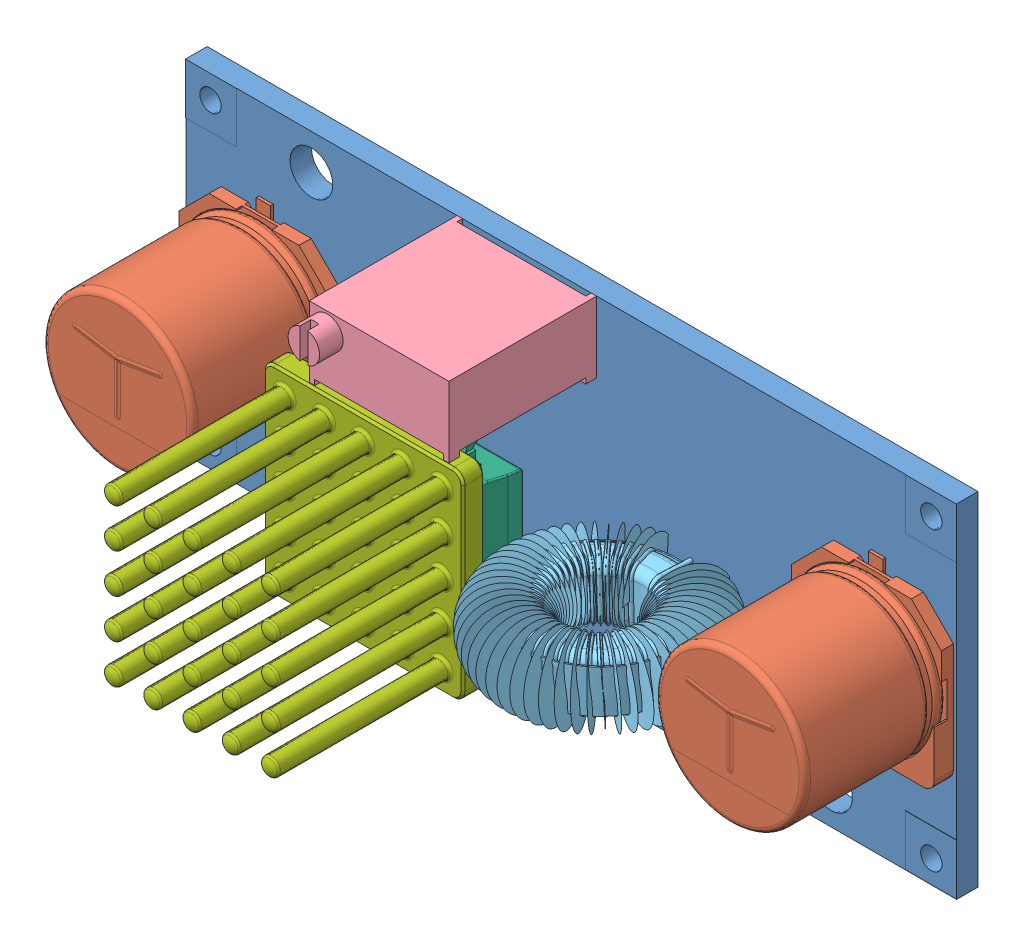
SolidWorks assembly XL4015 DC-DC StepDown Assembly1, configuration Default. Lengths in mm.
Overall size (54 24 21.05).
9 component instances, 7 part files, 0 mates.
Components (placement in the parent):
- XL4015 DC-DC StepDown Assembly1.stp-1: XL4015 DC-DC StepDown Assembly1.stp [Default] at origin size (54 24 21.05)
  - SDown PCB.stp-1: SDown PCB.stp [Default] at (-18.1024 -0.1248 0) size (54 24 1.54)
  - CAPAE-D10.0x10.2.stp-1: CAPAE-D10.0x10.2.stp [Default] at (-39.4721 4.5252 1.45) x (0 -1 0) z (0 0 1) size (12 10.5 10.5)
  - CAPAE-D10.0x10.2.stp-2: CAPAE-D10.0x10.2.stp [Default] at (3.4279 4.5252 1.45) x (0 -1 0) z (0 0 1) size (12 10.5 10.5)
  - SC-76A.stp-1: SC-76A.stp [Default] at (-10.7903 -7.7821 1.5) size (2.7 1.45 1.15)
  - 3296W.stp-1: 3296W.stp [Default] at (-21.2124 9.4152 1.5) x (-1 0 0) z (0 0 1) size (9.78 4.96 14.9)
  - original.stp-1: original.stp [Default] at (-9.5918 -1.6589 7.9923) x (-0.004295 -0.999989 0.00187) z (-0.998785 0.004198 -0.049105) size (5.4 14.32 14.64)
  - TO263-5-1.stp-1: TO263-5-1.stp [Default] at (-26.3572 -5.9186 1.4654) x (-1 0 0) z (0 0.006883 0.999976) size (9.83 14.6 4.22)
  - Enzotech-BMR-C1.stp-1: Enzotech-BMR-C1.stp [Default] at (-26.7842 -4.718 5.8987) x (1 0 0) z (0 -1 0) size (14 14 14)
